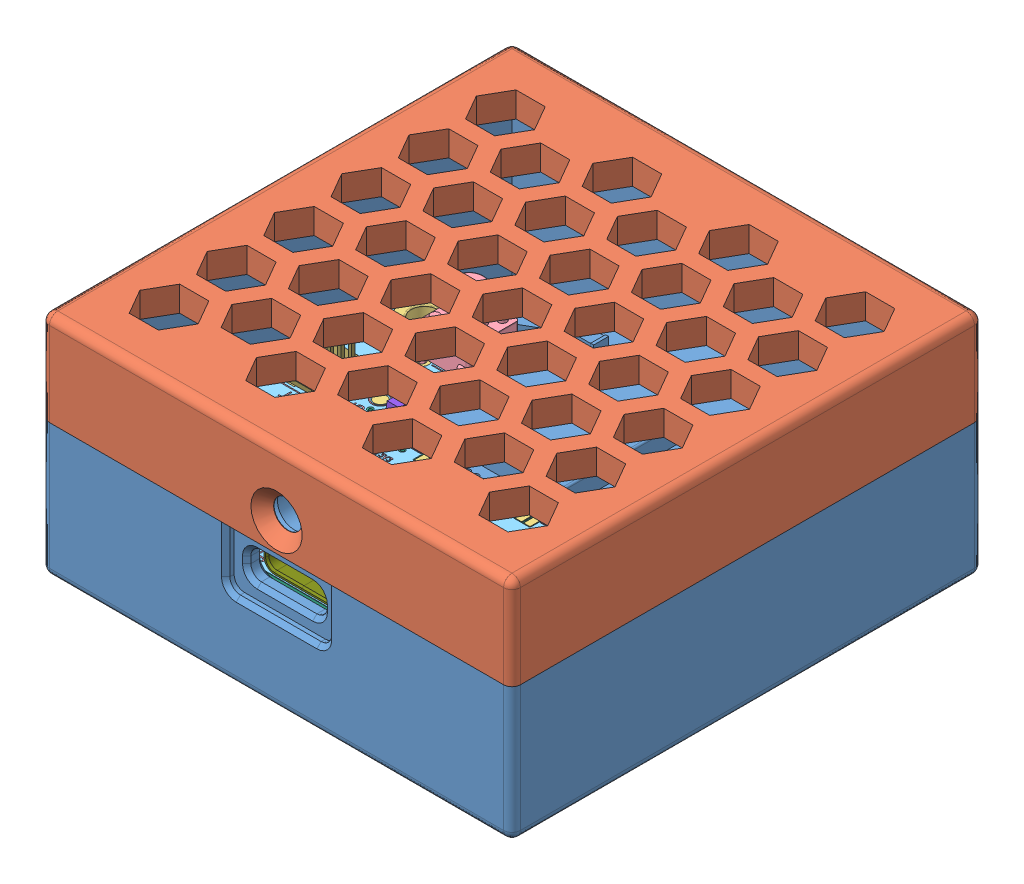
SolidWorks assembly Assem1, configuration Default. Lengths in mm.
Overall size (56 27 56).
52 component instances, 24 part files, 26 mates.
Components (placement in the parent):
- case-1: case [Default] at (-21.1368 5.0179 9.443) size (56 24 56)
- lid-1: lid [Default] at (-21.1368 20.0179 9.443) x (-1 0 0) z (0 0 1) size (56 11 56)
- UWBkit_minimal-1: UWBkit_minimal [Default] at (-172.7818 2.0179 -67.157) x (1 0 0) z (0 1 0) size (49.01 48.45 15.4)
  - UWBkit_minimal.step-1: UWBkit_minimal.step [Default] at origin size (49.01 48.45 15.4)
    - LED_0603_1608Metric.step-1: LED_0603_1608Metric.step [Default] at (168.7 -85.925 1.595) x (0 -1 0) z (0 0 1) size (1.6 0.8 1.1)
    - SW_PUSH_6mm_H7.3mm.step-1: SW_PUSH_6mm_H7.3mm.step [Default] at (139.45 -64.15 1.595) x (0 -1 0) z (0 0 1) size (7.17 6 10.8)
    - SOT-23-5.step-1: SOT-23-5.step [Default] at (141 -86.775 1.595) x (-1 0 0) z (0 0 1) size (2.8 2.9 1.55)
    - R_0603_1608Metric.step-1: R_0603_1608Metric.step [Default] at (165.5 -82.3 1.595) x (0 1 0) z (0 0 1) size (1.6 0.8 0.45)
    - R_0603_1608Metric.step-2: R_0603_1608Metric.step [Default] at (135.9 -83.2 1.595) x (0 -1 0) z (0 0 1) size (1.6 0.8 0.45)
    - R_0603_1608Metric.step-3: R_0603_1608Metric.step [Default] at (163.9 -82.3 1.595) x (0 1 0) z (0 0 1) size (1.6 0.8 0.45)
    - SOT-23.step-1: SOT-23.step [Default] at (168.1 -68.7 1.595) x (0 1 0) z (0 0 1) size (2.5 3 1.2)
    - CP_EIA-3216-18_Kemet-A.step-1: CP_EIA-3216-18_Kemet-A.step [Default] at (139.6 -77.2775 1.595) x (0 -1 0) z (0 0 1) size (3.2 1.6 1.8)
    - L_0805_2012Metric.step-1: L_0805_2012Metric.step [Default] at (137.8 -86.8 1.595) x (0 1 0) z (0 0 1) size (2 1.25 1.25)
    - C_0603_1608Metric.step-1: C_0603_1608Metric.step [Default] at (139.8 -73.325 1.595) x (0 1 0) z (0 0 1) size (1.6 0.8 0.8)
    - PinSocket_1x02_P2.54mm_Vertical.step-1: PinSocket_1x02_P2.54mm_Vertical.step [Default] at (142.275 -99 1.595) x (0 -1 0) z (0 0 1) size (2.54 5.08 11.6)
    - R_0603_1608Metric.step-4: R_0603_1608Metric.step [Default] at (167.9 -65.8 1.595) x (-1 0 0) z (0 0 1) size (1.6 0.8 0.45)
    - C_0603_1608Metric.step-2: C_0603_1608Metric.step [Default] at (146 -86.8 1.595) x (0 -1 0) z (0 0 1) size (1.6 0.8 0.8)
    - PinHeader_2x05_P1.27mm_Vertical_SMD.step-1: PinHeader_2x05_P1.27mm_Vertical_SMD.step [Default] at (130.8 -78 1.595) x (-1 0 0) z (0 0 1) size (5.57 6.35 4.4)
    - R_0603_1608Metric.step-5: R_0603_1608Metric.step [Default] at (167.8 -75.7 1.595) x (0 1 0) z (0 0 1) size (1.6 0.8 0.45)
    - SOT-23.step-2: SOT-23.step [Default] at (164.5 -68.7 1.595) x (0 1 0) z (0 0 1) size (2.5 3 1.2)
    - PinHeader_1x02_P2.54mm_Vertical.step-1: PinHeader_1x02_P2.54mm_Vertical.step [Default] at (130.8 -89.325 1.595) size (2.54 5.08 11.54)
    - R_0603_1608Metric.step-6: R_0603_1608Metric.step [Default] at (164.8 -75.7 1.595) x (0 1 0) z (0 0 1) size (1.6 0.8 0.45)
    - SOT-23-3.step-1: SOT-23-3.step [Default] at (143.025 -95 1.595) x (0 -1 0) z (0 0 1) size (2.5 3 1.2)
    - PinSocket_1x04_P2.54mm_Vertical.step-1: PinSocket_1x04_P2.54mm_Vertical.step [Default] at (172.7 -79.745 1.595) x (-1 0 0) z (0 0 1) size (2.54 10.16 11.6)
    - R_0603_1608Metric.step-7: R_0603_1608Metric.step [Default] at (164.7 -65.8 1.595) size (1.6 0.8 0.45)
    - LED_0603_1608Metric.step-2: LED_0603_1608Metric.step [Default] at (163.9 -85.925 1.595) x (0 -1 0) z (0 0 1) size (1.6 0.8 1.1)
    - SOT-23.step-3: SOT-23.step [Default] at (139.025 -95 1.595) x (0 -1 0) z (0 0 1) size (2.5 3 1.2)
    - R_0603_1608Metric.step-8: R_0603_1608Metric.step [Default] at (166.3 -75.7 1.595) x (0 1 0) z (0 0 1) size (1.6 0.8 0.45)
    - SOT-23-5.step-2: SOT-23-5.step [Default] at (141.025 -90.6 1.595) x (-1 0 0) z (0 0 1) size (2.8 2.9 1.55)
    - R_0603_1608Metric.step-9: R_0603_1608Metric.step [Default] at (167.9 -64.1 1.595) size (1.6 0.8 0.45)
    - USB_C_Receptacle_GCT_USB4105-xx-A_16P_TopMnt_Horizontal.step-1: USB_C_Receptacle_GCT_USB4105-xx-A_16P_TopMnt_Horizontal.step [Default] at (151.625 -97.94 1.595) size (8.94 7.78 4.26)
    - R_0603_1608Metric.step-10: R_0603_1608Metric.step [Default] at (155.825 -90.6 1.595) x (0 1 0) z (0 0 1) size (1.6 0.8 0.45)
    - C_0603_1608Metric.step-3: C_0603_1608Metric.step [Default] at (144.1 -86.8 1.595) x (0 -1 0) z (0 0 1) size (1.6 0.8 0.8)
    - R_0603_1608Metric.step-11: R_0603_1608Metric.step [Default] at (167.11 -82.3 1.595) x (0 1 0) z (0 0 1) size (1.6 0.8 0.45)
    - C_0603_1608Metric.step-4: C_0603_1608Metric.step [Default] at (135.9 -86.8 1.595) x (0 -1 0) z (0 0 1) size (1.6 0.8 0.8)
    - LED_0603_1608Metric.step-3: LED_0603_1608Metric.step [Default] at (165.5 -85.925 1.595) x (0 -1 0) z (0 0 1) size (1.6 0.8 1.1)
    - LED_0603_1608Metric.step-4: LED_0603_1608Metric.step [Default] at (167.11 -85.925 1.595) x (0 -1 0) z (0 0 1) size (1.6 0.8 1.1)
    - SC-74-6_1.55x2.9mm_P0.95mm.step-1: SC-74-6_1.55x2.9mm_P0.95mm.step [Default] at (151.625 -90.6 1.595) x (-1 0 0) z (0 0 1) size (2.7 2.9 1.18)
    - R_0603_1608Metric.step-12: R_0603_1608Metric.step [Default] at (144.1 -90.6 1.595) x (0 1 0) z (0 0 1) size (1.6 0.8 0.45)
    - LED_0603_1608Metric.step-5: LED_0603_1608Metric.step [Default] at (137.8 -83.2 1.595) x (0 -1 0) z (0 0 1) size (1.6 0.8 1.1)
    - C_0603_1608Metric.step-5: C_0603_1608Metric.step [Default] at (158.325 -99.2 1.595) x (0 -1 0) z (0 0 1) size (1.6 0.8 0.8)
    - R_0603_1608Metric.step-13: R_0603_1608Metric.step [Default] at (164.7 -64.1 1.595) size (1.6 0.8 0.45)
    - R_0603_1608Metric.step-14: R_0603_1608Metric.step [Default] at (158.325 -96.1 1.595) x (0 1 0) z (0 0 1) size (1.6 0.8 0.45)
    - LED_RGB_Wuerth-PLCC4_3.2x2.8mm_150141M173100.step-1: LED_RGB_Wuerth-PLCC4_3.2x2.8mm_150141M173100.step [Default] at (166.3 -72.5 1.595) size (3.5 2.8 2.05)
    - DWM3001C.step-1: DWM3001C.step [Default] at (151.6 -66.71 2.595) size (19.13 27.1 3.2)
    - R_0603_1608Metric.step-15: R_0603_1608Metric.step [Default] at (168.7 -82.3 1.595) x (0 1 0) z (0 0 1) size (1.6 0.8 0.45)
    - R_0603_1608Metric.step-16: R_0603_1608Metric.step [Default] at (147.325 -90.6 1.595) x (0 1 0) z (0 0 1) size (1.6 0.8 0.45)
    - BatteryHolder_Keystone_1058_1x2032.step-1: BatteryHolder_Keystone_1058_1x2032.step [Default] at (151.625 -82.7 -0.085) x (1 0 0) z (0 0 -1) size (31.86 16 5.08)
    - UWBkit_minimal_pad.step-1: UWBkit_minimal_pad.step [Default] at origin size (47.72 38.11 1.59)
    - UWBkit_minimal_silkscreen.step-1: UWBkit_minimal_silkscreen.step [Default] at origin size (46.73 38.02 1.67)
    - UWBkit_minimal_soldermask.step-1: UWBkit_minimal_soldermask.step [Default] at origin size (49.01 39.11 1.62)
    - UWBkit_minimal_PCB.step-1: UWBkit_minimal_PCB.step [Default] at origin size (49 39.1 1.51)
Mates (geometry in assembly coordinates):
- Coincident1: coincident anti-aligned: plane of case-1 through (-21.1368 2.0179 9.443) normal (0 1 0); plane of UWBkit_minimal.step-1/UWBkit_minimal_PCB.step-1 through (-172.7618 2.0179 -67.157) normal (0 -1 0)
- Distance1: distance = 0.5 mm anti-aligned: plane of UWBkit_minimal.step-1/UWBkit_minimal_PCB.step-1 through (-45.6368 2.0179 33.443) normal (-1 0 0); plane of case-1 through (-46.1368 14.0179 34.443) normal (1 0 0)
- Coincident3: coincident anti-aligned: plane of case-1 through (-46.1368 14.0179 34.443) normal (0 0 -1); plane of UWBkit_minimal.step-1/UWBkit_minimal_PCB.step-1 through (2.3632 2.0179 34.443) normal (0 0 1)
- Coincident7: coincident: plane of case-1 through (-46.1368 14.0179 34.443) normal (0 0 -1); plane of UWBkit_minimal.step-2/UWBkit_minimal_PCB.step-1 through (2.3632 2.0179 34.443) normal (0 0 1)
- Distance2: distance = 0.5 mm: plane of UWBkit_minimal.step-2/UWBkit_minimal_PCB.step-1 through (-45.6368 2.0179 33.443) normal (-1 0 0); plane of case-1 through (-46.1368 14.0179 34.443) normal (1 0 0)
- Coincident9: coincident anti-aligned: plane of case-1 through (-21.1368 2.0179 9.443) normal (0 1 0); plane of UWBkit_minimal.step-2/UWBkit_minimal_PCB.step-1 through (-172.7618 2.0179 -67.157) normal (0 -1 0)
- Coincident10: coincident anti-aligned: plane of case-1 through (-21.1368 2.0179 9.443) normal (0 1 0); plane of UWBkit_minimal-1/UWBkit_minimal.step-1/UWBkit_minimal_PCB.step-1 through (-172.7818 2.0179 -67.157) normal (0 -1 0)
- Concentric1: concentric anti-aligned: cylinder of case-1 through (-0.1568 -12.639 -1.157) axis (0 1 0) radius 2; cylinder of UWBkit_minimal-1/UWBkit_minimal.step-1/UWBkit_minimal_pad.step-1 through (-0.1568 1.9719 -1.157) axis (0 -1 0) radius 1.575
- Parallel1: parallel anti-aligned: plane of case-1 through (-46.1368 14.0179 34.443) normal (0 0 -1); plane of UWBkit_minimal-1/UWBkit_minimal.step-1/UWBkit_minimal_PCB.step-1 through (2.3432 2.0179 34.443) normal (0 0 1)
- Parallel2: parallel aligned: line of case-1 through (4.2632 9.0179 -16.957) axis (-1 0 0); line of oled-1 through (-8.6368 15.8179 4.043) axis (-1 0 0)
- Parallel3: parallel anti-aligned: plane of lid-1 through (-21.1368 20.0179 9.443) normal (0 1 0); plane of oled-1 through (-21.1368 15.8179 17.543) normal (0 -1 0)
- Distance3: distance = 14.1 mm anti-aligned: plane of oled-1 through (-33.6368 17.0179 31.043) normal (-1 0 0); plane of lid-1 through (-47.7368 17.0179 36.043) normal (1 0 0)
- Distance5: distance = 5 mm anti-aligned: plane of oled-1 through (-33.6368 17.0179 31.043) normal (0 0 1); plane of lid-1 through (5.4632 17.0179 36.043) normal (0 0 -1)
- Coincident16: coincident anti-aligned: plane of lid-1 through (-21.1368 17.0179 9.443) normal (0 -1 0); plane of oled-1 through (-21.1368 17.0179 17.543) normal (0 1 0)
- Distance6: distance = 0 mm aligned: plane of lid-1 through (-49.1368 9.0179 37.443) normal (-1 0 0); plane of case-1 through (-49.1368 14.0179 34.443) normal (-1 0 0)
- Distance7: distance = 0 mm aligned: plane of lid-1 through (6.8632 9.0179 37.443) normal (0 0 1); plane of case-1 through (-46.1368 14.0179 37.443) normal (0 0 1)
- LimitDistance1: limit distance = 0 mm anti-aligned: plane of lid-1 through (-21.1368 9.0179 9.443) normal (0 -1 0); plane of case-1 through (-21.1368 9.0179 9.443) normal (0 1 0)
- Distance10: distance = 0 mm aligned: plane of lid-1 through (-41.7368 26.0179 25.143) normal (-1 0 0); plane of oled_holder-1 through (-41.7368 26.0179 33.143) normal (-1 0 0)
- LimitDistance2: limit distance = 0 mm anti-aligned: plane of lid-1 through (-21.1368 26.0179 9.443) normal (0 -1 0); plane of oled_holder-1 through (-21.1368 26.0179 17.543) normal (0 1 0)
- Coincident24: coincident anti-aligned: plane of lid-1 through (-21.1368 26.0179 9.443) normal (0 -1 0); plane of oled_holder_part-2 through (-6.5368 76.0179 5.943) normal (0 1 0)
- Coincident25: coincident anti-aligned: plane of lid-1 through (-0.5368 23.0179 1.943) normal (-1 0 0); plane of oled_holder_part-2 through (-0.5368 76.0179 9.943) normal (1 0 0)
- Coincident26: coincident anti-aligned: plane of lid-1 through (-8.5368 23.0179 1.943) normal (0 0 1); plane of oled_holder_part-2 through (-12.5368 76.0179 1.943) normal (0 0 -1)
- Coincident27: coincident anti-aligned: plane of lid-1 through (-21.1368 26.0179 9.443) normal (0 -1 0); plane of oled_holder_part-1 through (-35.7368 76.0179 5.943) normal (0 1 0)
- Coincident29: coincident anti-aligned: plane of lid-1 through (-41.7368 23.0179 1.943) normal (1 0 0); plane of oled_holder_part-1 through (-41.7368 76.0179 1.943) normal (-1 0 0)
- Coincident30: coincident anti-aligned: plane of lid-1 through (-33.7368 23.0179 1.943) normal (0 0 1); plane of oled_holder_part-1 through (-29.7368 76.0179 1.943) normal (0 0 -1)
- Distance13: distance = 0 mm aligned: plane of lid-1 through (-41.7368 26.0179 33.143) normal (0 0 1); plane of oled_holder-1 through (-41.7368 26.0179 33.143) normal (0 0 1)
